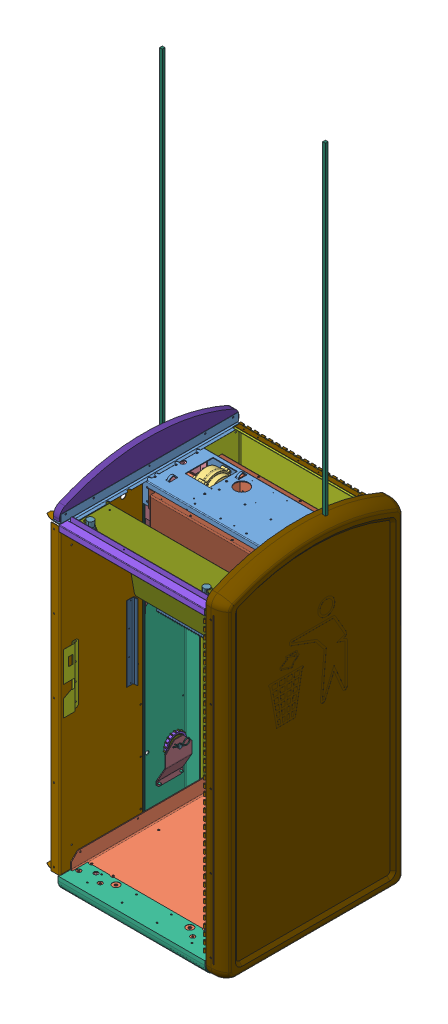
SolidWorks assembly Corrigé_BB3_Assy_Meca_3D_2, configuration Défaut. Lengths in mm.
Overall size (675.82 1282.03 663.93).
120 component instances, 56 part files, 9 mates.
Components (placement in the parent):
- BB3_Chassis-1: BB3_Chassis [Défaut] at (-140.0351 388.7943 -82.8142) size (675.82 1282.03 663.93)
  - TopCrossmember_Rev2-1: TopCrossmember_Rev2 [Default] at (20.5473 102.5902 0) size (635 86.99 210.82)
  - TopCrossMotorBrkt_Rev3-1: TopCrossMotorBrkt_Rev3 [Défaut] at (-101.9976 61.051 0) size (152.4 200.54 205.51)
  - Moto_Reducteur_011_562_1_216-1: Moto_Reducteur_011_562_1_216 [Default] at (192.9322 74.2423 -36.8146) x (0 -0.000019 -1) z (-1 0 0) size (114.3 226.4 239.81)
  - TopCrossBearingBrkt_Rev1-1: TopCrossBearingBrkt_Rev1 [Défaut] at (-246.0257 61.051 0) size (25.4 73.66 205.51)
  - TopCrossBearingBrkt_Rev1-2: TopCrossBearingBrkt_Rev1 [Défaut] at (287.1203 61.051 0) x (-1 0 0) z (0 0 -1) size (25.4 73.66 205.51)
  - Chassis_Coussinet-1: Chassis_Coussinet [Default] at (-247.5497 60.2788 -36.8146) x (0 -0.995993 0.089436) z (0 0.089436 0.995993) size (28.27 19.05 28.27)
  - Chassis_Coussinet-2: Chassis_Coussinet [Default] at (288.6443 60.2788 -36.8146) x (0 0.997938 0.064185) z (0 -0.064185 0.997938) size (28.27 19.05 28.27)
  - Chassis_Support_Moteur-1: Chassis_Support_Moteur [Défaut] at (-296.9017 100.6288 0.0002) x (0 0 1) z (0 1 0) size (205.51 54 1127)
  - Chassis_Support_Moteur-2: Chassis_Support_Moteur [Défaut] at (337.9963 100.6288 0.0002) x (0 0 -1) z (0 1 0) size (205.51 54 1127)
  - Chassis_Panneau_Arriere-2: Chassis_Panneau_Arriere [Défaut] at (20.5983 -479.4712 -246.619) x (0 0 1) z (0 1 0) size (164.98 667 1155.29)
  - Chassis_Support_Batterie-2: Chassis_Support_Batterie [Défaut] at (20.5983 -270.8192 -242.544) x (0 0 1) z (-1 0 0) size (116.32 446 529)
  - Chassis_Support_Moteur_Devant_Gauche-2: Chassis_Support_Moteur_Devant_Gauche [Défaut] at (-249.8894 -442.8187 130.7585) x (0 0 -1) z (0 1 0) size (329.85 66 1105)
  - Chassis_Positionnement_Emetteur_Recepteur_Gauche-2: Chassis_Positionnement_Emetteur_Recepteur_Gauche [Défaut] at (-222.4622 -381.8185 156.8606) x (1 0 0) z (0 -1 0) size (22.1 48.5 273)
  - Chassis_Support_Moteur_Devant_Droite-1: Chassis_Support_Moteur_Devant_Droite [Défaut] at (290.9839 -442.8187 130.7585) x (0 0 -1) z (0 -1 0) size (329.85 66 1105)
  - Chassis_Positionnement_Emetteur_Recepteur_Droite-1: Chassis_Positionnement_Emetteur_Recepteur_Droite [Défaut] at (263.5568 -381.8185 156.8606) x (-1 0 0) z (0 1 0) size (22.1 48.5 273)
  - Chassis_Support_Pignon_bas-1: Chassis_Support_Pignon_bas [Défaut] at (305.4963 -865.3715 -39.8528) x (-1 0 0) z (0 0 1) size (35.2 151.29 95)
  - Chassis_Axe_Pignon_Bas-1: Chassis_Axe_Pignon_Bas [Défaut] at (340.9963 -816.3715 -39.8528) x (-1 0 0) z (0 -0.052233 -0.998635) size (48.6 15.9 15.9)
  - Chassis_Goupille_Axe_Pignon_bas-1: Chassis_Goupille_Axe_Pignon_bas [Défaut] at (300.5463 -817.6251 -63.8201) x (0 0.052233 0.998635) z (1 0 0) size (60.5 23 3)
  - Chassis_Support_Pignon_bas-2: Chassis_Support_Pignon_bas [Défaut] at (-264.4017 -865.3715 -39.8528) x (1 0 0) z (0 0 -1) size (35.2 151.29 95)
  - Chassis_Axe_Pignon_Bas-2: Chassis_Axe_Pignon_Bas [Défaut] at (-299.9017 -816.3715 -39.8528) x (1 0 0) z (0 0.31653 0.948583) size (48.6 15.9 15.9)
  - Chassis_Goupille_Axe_Pignon_bas-2: Chassis_Goupille_Axe_Pignon_bas [Défaut] at (-259.4517 -808.7748 -17.0869) x (0 -0.31653 -0.948583) z (1 0 0) size (60.5 23 3)
  - Chassis_Plaque_Haute-1: Chassis_Plaque_Haute [Défaut] at (20.4963 92.768 412.6062) x (0 0 -1) z (1 0 0) size (278.51 354.1 562.7)
  - Chassis_Renfort-1: Chassis_Renfort [Défaut] at (20.5463 -1018.8712 0.0002) x (0 0 1) z (-1 0 0) size (199.51 39 641)
  - Chassis_Charniere_Photovoltaique-1: Chassis_Charniere_Photovoltaique [Défaut] at (20.5983 134.4053 -220.1468) x (0 0 -1) z (1 0 0) size (21.77 6 520)
  - Chassis_Equerre_Haute-1: Chassis_Equerre_Haute [Défaut] at (-246.1446 112.2812 81.6782) x (1 0 0.000001) z (-0.000001 0 1) size (44 37.45 648)
  - Chassis_Equerre_Haute-2: Chassis_Equerre_Haute [Défaut] at (287.2893 112.2812 81.6751) x (-1 0 -0.000168) z (0.000168 0 -1) size (44 37.45 648)
  - Chassis_Repose_Bac_Dechets-1: Chassis_Repose_Bac_Dechets [Défaut] at (20.4963 -992.8728 80.2436) x (0 -0.000001 1) z (-1 0 0) size (641.73 77 529)
  - Chassis_Semelle-1: Chassis_Semelle [Défaut] at (20.4963 -1034.3925 80.4561) x (1 0 0) z (0 -0.000001 1) size (404.15 56 558)
  - Chassis_Repose_Pied-1: Chassis_Repose_Pied [Défaut] at (-187.0037 -1049.3185 336.4561) x (1 0 0) z (0 -0.000001 1) size (94 52.5 63.3)
  - Chassis_Repose_Pied-2: Chassis_Repose_Pied [Défaut] at (-187.0037 -1049.3182 -175.5439) x (1 0 0) z (0 -0.000001 1) size (94 52.5 63.3)
  - Chassis_Repose_Pied-3: Chassis_Repose_Pied [Défaut] at (227.9963 -1049.3182 -175.5439) x (1 0 0) z (0 -0.000001 1) size (94 52.5 63.3)
  - Chassis_Repose_Pied-4: Chassis_Repose_Pied [Défaut] at (227.9963 -1049.3185 336.4561) x (1 0 0) z (0 -0.000001 1) size (94 52.5 63.3)
  - Chassis_Repose_Pied_Insert-1: Chassis_Repose_Pied_Insert [Défaut] at (-187.0037 -1050.3185 336.4561) x (0 1 0.000001) z (0.428959 -0.000001 0.903324) size (14.3 17.5 17.5)
  - Chassis_Repose_Pied_Insert-2: Chassis_Repose_Pied_Insert [Défaut] at (227.9963 -1050.3185 336.4561) x (0 1 0.000001) z (0.384049 -0.000001 0.923313) size (14.3 17.5 17.5)
  - Chassis_Repose_Pied_Insert-3: Chassis_Repose_Pied_Insert [Défaut] at (227.9963 -1050.3182 -175.5439) x (0 1 0.000001) z (-0.000001 -0.000001 1) size (14.3 17.5 17.5)
  - Chassis_Repose_Pied_Insert-4: Chassis_Repose_Pied_Insert [Défaut] at (-187.0037 -1050.3182 -175.5439) x (0 1 0.000001) z (-0.000001 -0.000001 1) size (14.3 17.5 17.5)
  - Chassis_Repose_Pied_Insert-5: Chassis_Repose_Pied_Insert [Défaut] at (-114.0037 -995.8185 336.4561) x (0 -1 -0.000001) z (0.798225 0 0.602359) size (14.3 17.5 17.5)
  - Chassis_Repose_Pied_Insert-6: Chassis_Repose_Pied_Insert [Défaut] at (154.9963 -995.8185 336.4561) x (0 -1 -0.000001) z (0.000001 -0.000001 1) size (14.3 17.5 17.5)
  - Chassis_Repose_Pied_Insert-7: Chassis_Repose_Pied_Insert [Défaut] at (-114.0037 -995.8182 -175.5439) x (0 -1 -0.000001) z (0.000001 -0.000001 1) size (14.3 17.5 17.5)
  - Chassis_Repose_Pied_Insert-8: Chassis_Repose_Pied_Insert [Défaut] at (154.9963 -995.8182 -175.5439) x (0 -1 -0.000001) z (0.000001 -0.000001 1) size (14.3 17.5 17.5)
  - Chassis_Dessous_Avant_Porte-1: Chassis_Dessous_Avant_Porte [Défaut] at (20.4963 -992.8728 80.2436) x (0 -0.000001 1) z (-1 0 0) size (98 53.79 536)
  - Chassis_Serrure-1: Chassis_Serrure [Défaut] at (-243.4017 -382.964 366.4072) x (1 0 0) z (0 1 0) size (10.5 63.82 216)
  - Chassis_Equerre_Face-1: Chassis_Equerre_Face [Défaut] at (20.4963 111.0096 411.9878) x (0 0 1) z (-1 0 0) size (32.2 41.42 529)
  - Chassis_Charniere_Support_Moteur_Devant_Droite-1: Chassis_Charniere_Support_Moteur_Devant_Droite [Défaut] at (260.2718 -465.3185 388.412) x (0 0 1) z (0 -1 0) size (21.77 6 1066)
  - Chassis_Serrure_Cle-1: Chassis_Serrure_Cle [Défaut] at (-191.3537 126.1269 363.7894) x (0 1 0) z (-1 0 0) size (41.58 38.56 38.97)
    - Chassis_Serrure_Came-1: Chassis_Serrure_Came [Défaut] at (-18.246 14.5659 16.3878) x (0 -1 0) z (1 0 0) size (12.45 12.01 13.54)
    - Chassis_Serrure_Rondelle_Ecrou-1: Chassis_Serrure_Rondelle_Ecrou [Défaut] at (-31.074 17.7899 -9.8703) x (0 0.096744 0.995309) z (-1 0 0) size (35.31 35.31 0.64)
    - Chassis_Serrure_Ecrou_Hex-1: Chassis_Serrure_Ecrou_Hex [Défaut] at (-26.3115 -31.157 8.2014) x (0 0 1) z (-1 0 0) size (33 28.58 4.76)
    - Chassis_Serrure_Insert_Cle-1: Chassis_Serrure_Insert_Cle [Défaut] at (26.379 -212.8643 14.6) x (-1 0 0) z (0 0 -1) size (23.33 15.95 15.95)
    - Chassis_Serrure_Support-1: Chassis_Serrure_Support [Défaut] at (-26.6815 11.1833 12.473) x (-1 0 0) z (0 -1 0) size (41.46 28.7 28.7)
    - Chassis_Serrure_Ressort-1: Chassis_Serrure_Ressort [Défaut] at (-1.4058 10.243 9.1044) x (0 0 -1) z (1 0 0) size (21.49 4.59 4.57)
    - Chassis_Serrure_Pene-1: Chassis_Serrure_Pene [Défaut] at (1.0072 5.2825 -10.1896) x (0 -0.999973 -0.007317) z (-1 0 0) size (16.91 23.47 9.63)
  - Chassis_Serrure_Cle-2: Chassis_Serrure_Cle [Défaut] at (232.3463 126.1269 341.4229) x (0 1 0) z (1 0 0) size (41.58 38.56 38.97)
    - Chassis_Serrure_Came-1: Chassis_Serrure_Came [Défaut] at (-18.246 14.5659 16.3878) x (0 -1 0) z (1 0 0) size (12.45 12.01 13.54)
    - Chassis_Serrure_Rondelle_Ecrou-1: Chassis_Serrure_Rondelle_Ecrou [Défaut] at (-31.074 17.7899 -9.8703) x (0 0.096744 0.995309) z (-1 0 0) size (35.31 35.31 0.64)
    - Chassis_Serrure_Ecrou_Hex-1: Chassis_Serrure_Ecrou_Hex [Défaut] at (-26.3115 -31.157 8.2014) x (0 0 1) z (-1 0 0) size (33 28.58 4.76)
    - Chassis_Serrure_Insert_Cle-1: Chassis_Serrure_Insert_Cle [Défaut] at (26.379 -212.8643 14.6) x (-1 0 0) z (0 0 -1) size (23.33 15.95 15.95)
    - Chassis_Serrure_Support-1: Chassis_Serrure_Support [Défaut] at (-26.6815 11.1833 12.473) x (-1 0 0) z (0 -1 0) size (41.46 28.7 28.7)
    - Chassis_Serrure_Ressort-1: Chassis_Serrure_Ressort [Défaut] at (-1.4058 10.243 9.1044) x (0 0 -1) z (1 0 0) size (21.49 4.59 4.57)
    - Chassis_Serrure_Pene-1: Chassis_Serrure_Pene [Défaut] at (1.0072 5.2825 -10.1896) x (0 -0.999973 -0.007317) z (-1 0 0) size (16.91 23.47 9.63)
  - Tombstone_Rev1-1: Tombstone_Rev1 [Default] at (288.5894 129.5652 81.0473) x (1 0 0.000168) z (-0.000168 0 1) size (22.23 105.62 654.05)
  - Tombstone_Rev1-2: Tombstone_Rev1 [Default] at (-247.4446 129.5652 82.3062) x (-1 0 -0.000001) z (0.000001 0 -1) size (22.23 105.62 654.05)
  - SideSkin_Rev1-1: SideSkin_Rev1 [Default] at (-317.3073 -1045.6118 82.3061) x (-1 0 -0.000001) z (0.000001 0 -1) size (69.87 1274.83 660.4) (hidden)
  - SideSkin_Rev1-2: SideSkin_Rev1 [Default] at (358.4521 -1045.6118 81.059) x (1 0 0.000168) z (-0.000168 0 1) size (69.87 1274.83 660.4)
  - Chassis_Interieur_Cache_Chaine-1: Chassis_Interieur_Cache_Chaine [Défaut] at (-242.9017 -763.8184 0) x (0 -0.000001 1) z (-1 0 0) size (249 989 21) (hidden)
  - Chassis_Interieur_Cache_Chaine-2: Chassis_Interieur_Cache_Chaine [Défaut] at (283.9963 -763.8185 0.0002) x (0 0 -1) z (1 0 0) size (249 989 21)
  - Chassis_Bac_Dechets-1: Chassis_Bac_Dechets [Défaut] at (19.5983 -711.9931 65.1059) x (-1 0 0) z (0 0.000001 -1) size (517 387.96 620.45) (hidden)
- BB3_Axe_Moteur-1: BB3_Axe_Moteur [Défaut] at (-118.6236 449.4588 -117.6952) size (601.11 82.55 82.55)
  - TransmissionShaft_Rev1-1: TransmissionShaft_Rev1 [Défaut] at (-0.7672 -0.3857 -1.9336) size (596.9 18.75 19.05)
  - CounterDisc_Rev1-1: CounterDisc_Rev1 [Défaut] at (188.8209 -0.3857 -1.9336) size (0.91 82.55 82.55)
  - Pignon_Haut-1: Pignon_Haut [Défaut] at (-297.0312 -0.3857 -1.9336) x (0 0 1) z (-1 0 0) (suppressed, hidden)
  - Pignon_Haut-2: Pignon_Haut [Défaut] at (294.0828 -0.3857 -1.9336) x (0 0 -1) z (1 0 0) (suppressed, hidden)
  - SHAFT_COLLAR_MCMASTER_6166K28-1: SHAFT_COLLAR_MCMASTER_6166K28 [Défaut] at (181.6772 -0.3857 -1.9336) size (14.29 38.1 38.1)
  - TRANSMISSION_KEY_MC_98870A140-1: TRANSMISSION_KEY_MC_98870A140 [Défaut] at (-285.8172 18.6654 -1.9336) x (-1 0 0) z (0 0 1) size (25.4 4.76 4.76)
  - TRANSMISSION_KEY_MC_98870A140-2: TRANSMISSION_KEY_MC_98870A140 [Défaut] at (284.2828 18.6654 -1.9336) x (-1 0 0) z (0 0 1) size (25.4 4.76 4.76)
  - TRANSMISSION_KEY_MC_98870A190-1: TRANSMISSION_KEY_MC_98870A190 [Défaut] at (-155.0672 18.6654 -1.9336) x (-1 0 0) z (0 0 1) size (63.5 4.76 4.76)
  - PURPLE_IGUS-1: PURPLE_IGUS [Défaut] at (191.2568 -0.3857 -1.9336) x (0 0.381849 -0.924225) z (0 0.924225 0.381849) size (28.27 19.05 28.27)
  - BB3_Pignon_Cylindre_Primitif-1: BB3_Pignon_Cylindre_Primitif [Défaut] at (-295.6312 -0.3857 -1.9336) x (0 0 -1) z (1 0 0) size (73.14 73.14 10)
  - BB3_Pignon_Cylindre_Primitif-2: BB3_Pignon_Cylindre_Primitif [Défaut] at (295.4828 -0.3857 -1.9336) x (0 0 -1) z (1 0 0) size (73.14 73.14 10)
  - Pignon_Haut-3: Pignon_Haut [Défaut] at (-297.0312 -0.3857 -1.9336) x (0 0 1) z (-1 0 0)
  - Pignon_Haut-4: Pignon_Haut [Défaut] at (296.8828 -0.3857 -1.9336) x (0 0 -1) z (1 0 0)
- BB3_Rame_Compacteur-1: BB3_Rame_Compacteur [Défaut] at (-143.8198 251.6092 -80.1568) size (627.3 1739.7 268.31)
  - Compacteur_Rame-1: Compacteur_Rame [Défaut] at (24.383 25.4321 -2.9042) size (505.8 287.44 265.81)
  - Compacteur_Flasque-1: Compacteur_Flasque [Défaut] at (23.883 58.9321 129.5958) x (-1 0 0) z (0 0 -1) size (481.4 343 21.8)
  - Compacteur_Flasque-2: Compacteur_Flasque [Défaut] at (24.883 58.9321 -135.4042) size (481.4 343 21.8)
  - Compacteur_Guide_Droit-1: Compacteur_Guide_Droit [Défaut] at (297.583 154.6611 -2.9042) x (0 0 1) z (0 -1 0) size (185.61 92.3 356)
  - Compacteur_Guide_Gauche-1: Compacteur_Guide_Gauche [Défaut] at (-250.117 154.6611 -2.9042) x (0 0 -1) z (0 -1 0) size (185.61 93.6 356)
  - Compacteur_Guide_Patin-1: Compacteur_Guide_Patin [Défaut] at (-270.917 -23.3389 -95.7102) x (-1 0 0) z (0 0 -1) size (38 350 6.7)
  - Compacteur_Guide_Patin-2: Compacteur_Guide_Patin [Défaut] at (-270.917 -23.3389 89.9018) size (38 350 6.7)
  - Compacteur_Guide_Patin-3: Compacteur_Guide_Patin [Défaut] at (318.383 -23.3389 89.9018) size (38 350 6.7)
  - Compacteur_Guide_Patin-4: Compacteur_Guide_Patin [Défaut] at (318.383 -23.3389 -95.7102) x (-1 0 0) z (0 0 -1) size (38 350 6.7)
  - BB3_Coulissant_Vertical_Cremaillere-1: BB3_Coulissant_Vertical_Cremaillere [Défaut] at (-273.2835 838.3611 2.0958) x (-1 0 0) z (0 -1 0) size (10 10 1400)
  - BB3_Coulissant_Vertical_Cremaillere-2: BB3_Coulissant_Vertical_Cremaillere [Défaut] at (320.7496 838.3611 2.0958) x (1 0 0) z (0 1 0) size (10 10 1400)
- BB3_Pignon_Bas-1: BB3_Pignon_Bas [Défaut] at (-415.6548 -432.9543 -114.7035) x (0 0 -1) z (1 0 0) size (78.63 79.65 18.29)
  - Pignon_Bas-1: Pignon_Bas [Défaut] at (7.9635 5.3771 0) size (78.63 79.65 11.2)
  - Bearing_203KRR5-1: Bearing_203KRR5 [Défaut] at (7.9635 5.3771 0) x (0 0 -1) z (1 0 0) size (12 56.49 56.49)
    - Bearing_203KRR5_BE-1: Bearing_203KRR5_BE [Défaut] x (-1 0 0) z (0 -0.669852 0.742494) size (12 40 40)
    - Bearing_203KRR5_ER-1: Bearing_203KRR5_ER [Défaut] at (0 10.8207 9.7621) x (1 0 0) z (0 0.742494 0.669852) size (6 6 6)
    - Bearing_203KRR5_ER-2: Bearing_203KRR5_ER [Défaut] at (0 14.3789 -2.3734) x (1 0 0) z (0 0.986649 -0.162859) size (6 6 6)
    - Bearing_203KRR5_ER-3: Bearing_203KRR5_ER [Défaut] at (0 7.1095 -12.7217) x (1 0 0) z (0 0.487837 -0.872935) size (6 6 6)
    - Bearing_203KRR5_ER-4: Bearing_203KRR5_ER [Défaut] at (0 -5.5135 -13.4903) x (1 0 0) z (0 -0.378326 -0.925672) size (6 6 6)
    - Bearing_203KRR5_ER-5: Bearing_203KRR5_ER [Défaut] at (0 -13.9848 -4.1004) x (1 0 0) z (0 -0.959602 -0.28136) size (6 6 6)
    - Bearing_203KRR5_ER-6: Bearing_203KRR5_ER [Défaut] at (0 -11.9252 8.3772) x (1 0 0) z (0 -0.818278 0.574822) size (6 6 6)
    - Bearing_203KRR5_ER-7: Bearing_203KRR5_ER [Défaut] at (0 -0.8857 14.5466) x (1 0 0) z (0 -0.060774 0.998152) size (6 6 6)
  - Bearing_203KRR5_BI-1: Bearing_203KRR5_BI [Défaut] at (7.9635 5.3771 0) x (0 0 -1) z (1 0 0) size (18.29 24.43 24.43)
  - BB3_Pignon_Cylindre_Primitif-1: BB3_Pignon_Cylindre_Primitif [Défaut] at (7.9635 5.3771 1.4) size (73.14 73.14 10)
- BB3_Pignon_Bas-2: BB3_Pignon_Bas [Défaut] at (178.2592 -432.9543 -130.6306) x (0 0 1) z (-1 0 0) size (78.63 79.65 18.29)
  - Pignon_Bas-1: Pignon_Bas [Défaut] at (7.9635 5.3771 0) size (78.63 79.65 11.2)
  - Bearing_203KRR5-1: Bearing_203KRR5 [Défaut] at (7.9635 5.3771 0) x (0 0 -1) z (1 0 0) size (12 56.49 56.49)
    - Bearing_203KRR5_BE-1: Bearing_203KRR5_BE [Défaut] x (-1 0 0) z (0 -0.669852 0.742494) size (12 40 40)
    - Bearing_203KRR5_ER-1: Bearing_203KRR5_ER [Défaut] at (0 10.8207 9.7621) x (1 0 0) z (0 0.742494 0.669852) size (6 6 6)
    - Bearing_203KRR5_ER-2: Bearing_203KRR5_ER [Défaut] at (0 14.3789 -2.3734) x (1 0 0) z (0 0.986649 -0.162859) size (6 6 6)
    - Bearing_203KRR5_ER-3: Bearing_203KRR5_ER [Défaut] at (0 7.1095 -12.7217) x (1 0 0) z (0 0.487837 -0.872935) size (6 6 6)
    - Bearing_203KRR5_ER-4: Bearing_203KRR5_ER [Défaut] at (0 -5.5135 -13.4903) x (1 0 0) z (0 -0.378326 -0.925672) size (6 6 6)
    - Bearing_203KRR5_ER-5: Bearing_203KRR5_ER [Défaut] at (0 -13.9848 -4.1004) x (1 0 0) z (0 -0.959602 -0.28136) size (6 6 6)
    - Bearing_203KRR5_ER-6: Bearing_203KRR5_ER [Défaut] at (0 -11.9252 8.3772) x (1 0 0) z (0 -0.818278 0.574822) size (6 6 6)
    - Bearing_203KRR5_ER-7: Bearing_203KRR5_ER [Défaut] at (0 -0.8857 14.5466) x (1 0 0) z (0 -0.060774 0.998152) size (6 6 6)
  - Bearing_203KRR5_BI-1: Bearing_203KRR5_BI [Défaut] at (7.9635 5.3771 0) x (0 0 -1) z (1 0 0) size (18.29 24.43 24.43)
  - BB3_Pignon_Cylindre_Primitif-1: BB3_Pignon_Cylindre_Primitif [Défaut] at (7.9635 5.3771 1.4) size (73.14 73.14 10)
Mates (geometry in assembly coordinates):
- Coaxiale1: concentric anti-aligned: cylinder of BB3_Chassis-1/Chassis_Coussinet-1 through (-387.5848 449.0731 -119.6288) axis (1 0 0) radius 9.6139; cylinder of BB3_Axe_Moteur-1/TransmissionShaft_Rev1-1 through (179.0592 449.0731 -119.6288) axis (-1 0 0) radius 9.525
- Distance1: distance = 9.56 mm anti-aligned: plane of BB3_Axe_Moteur-1/Pignon_Haut-3 through (-397.1448 449.0731 -119.6288) normal (1 0 0); plane of BB3_Chassis-1/Chassis_Coussinet-1 through (-387.5848 449.0731 -119.6288) normal (-1 0 0)
- Coïncidente2: coincident aligned: plane of BB3_Chassis-1/Chassis_Panneau_Arriere-2; plane of BB3_Rame_Compacteur-1/Compacteur_Rame-1 through (-119.4368 277.0413 -83.061) normal (1 0 0)
- Coïncidente3: coincident anti-aligned: plane of BB3_Chassis-1/Chassis_Support_Moteur-1 through (-385.9368 -637.5769 -182.567) normal (0 0 1); plane of BB3_Rame_Compacteur-1/Compacteur_Guide_Patin-1 through (-414.7368 228.2703 -182.567) normal (0 0 -1)
- Distance2: distance = 12 mm aligned: plane of BB3_Rame_Compacteur-1/Compacteur_Flasque-2 through (-335.4368 482.0413 -215.561) normal (0 1 0); plane of BB3_Chassis-1/TopCrossmember_Rev2-1 through (-436.9878 494.0413 22.5958) normal (0 1 0)
- Coaxiale2: concentric anti-aligned: cylinder of BB3_Chassis-1/Chassis_Axe_Pignon_Bas-2 through (-417.6368 -427.5772 -122.667) axis (1 0 0) radius 6.25; cylinder of BB3_Pignon_Bas-1/Bearing_203KRR5_BI-1 through (-415.6548 -427.5772 -122.667) axis (-1 0 0) radius 6.5405
- Coïncidente5: coincident aligned: plane of BB3_Axe_Moteur-1/Pignon_Haut-3 through (-419.2548 469.8587 -119.6288) normal (-1 0 0); plane of BB3_Pignon_Bas-1/Pignon_Bas-1 through (-419.2548 -406.7916 -122.667) normal (-1 0 0)
- Coaxiale3: concentric anti-aligned: cylinder of BB3_Chassis-1/Chassis_Axe_Pignon_Bas-1 through (178.6612 -427.5772 -122.667) axis (-1 0 0) radius 6.25; cylinder of BB3_Pignon_Bas-2/Bearing_203KRR5_BI-1 through (178.2592 -427.5772 -122.667) axis (1 0 0) radius 6.5405
- Coïncidente6: coincident aligned: plane of BB3_Axe_Moteur-1/Pignon_Haut-4 through (181.8592 469.8587 -119.6288) normal (1 0 0); plane of BB3_Pignon_Bas-2/Pignon_Bas-1 through (181.8592 -406.7916 -122.667) normal (1 0 0)
